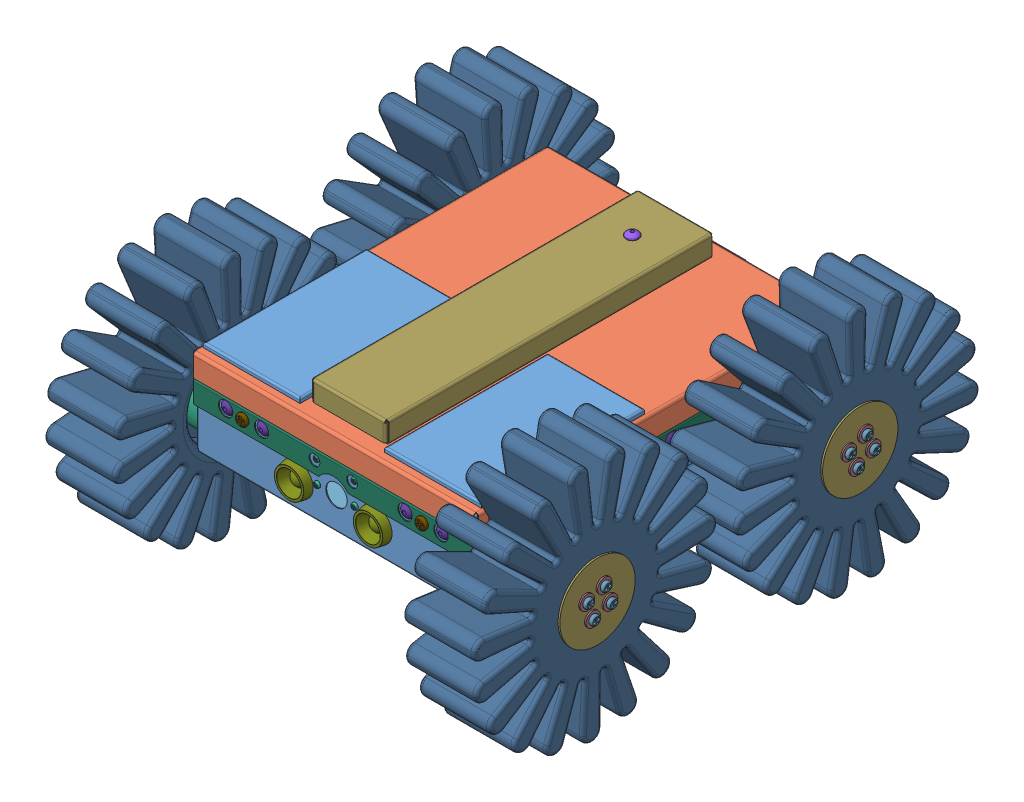
SolidWorks assembly GB0814, configuration Default. Lengths in mm. (continued)
Components (placement in the parent): (continued)
- wheel.assembly-2: wheel.assembly [Default] at (63.2286 -85.6639 -5.4063) x (0 0.437031 0.899447) z (-1 0 0) size (135.84 135.37 44.03)
  - wheel-1: wheel [Default] at (66.6468 86.2072 65.7286) size (135.84 135.37 40.29)
  - wheel.spacer-1: wheel.spacer [Default] at (66.6468 86.2072 79.7286) x (0.629376 -0.777101 0) z (-0.777101 -0.629376 0) size (21 1 21)
  - wheel.flap-1: wheel.flap [Default] at (66.6468 86.2072 106.7286) x (-0.999542 -0.030263 0) z (0 0 -1) size (42 42 1)
  - m3.washer-1: m3.washer [Default] at (69.6683 92.7975 107.5286) x (-0.923728 -0.383049 0) z (0 0 -1) size (8 8 0.8)
  - m3.washer-2: m3.washer [Default] at (60.0564 89.2288 107.5286) x (-0.923728 -0.383049 0) z (0 0 -1) size (8 8 0.8)
  - m3.washer-3: m3.washer [Default] at (63.6252 79.6169 107.5286) x (-0.923728 -0.383049 0) z (0 0 -1) size (8 8 0.8)
  - m3.washer-4: m3.washer [Default] at (73.2371 83.1856 107.5286) x (-0.923728 -0.383049 0) z (0 0 -1) size (8 8 0.8)
  - m3.screw.36mm-1: m3.screw.36mm [Default] at (73.2444 83.2034 107.5286) x (-0.923728 -0.383049 0) z (0 0 -1) size (5.42 5.42 38.08)
  - m3.screw.36mm-2: m3.screw.36mm [Default] at (63.6325 79.6346 107.5286) x (-0.923728 -0.383049 0) z (0 0 -1) size (5.42 5.42 38.08)
  - m3.screw.36mm-3: m3.screw.36mm [Default] at (69.6757 92.8153 107.5286) x (-0.923728 -0.383049 0) z (0 0 -1) size (5.42 5.42 38.08)
  - m3.screw.36mm-4: m3.screw.36mm [Default] at (60.0754 89.232 107.5286) x (-0.815437 0.578846 0) z (0 0 -1) size (5.42 5.42 38.08)
- wheel.assembly-3: wheel.assembly [Default] at (63.2286 -73.2341 108.359) x (0 0.131707 0.991289) z (-1 0 0) size (135.84 135.37 44.03)
  - wheel-1: wheel [Default] at (66.6468 86.2072 65.7286) size (135.84 135.37 40.29)
  - wheel.spacer-1: wheel.spacer [Default] at (66.6468 86.2072 79.7286) x (0.629376 -0.777101 0) z (-0.777101 -0.629376 0) size (21 1 21)
  - wheel.flap-1: wheel.flap [Default] at (66.6468 86.2072 106.7286) x (-0.999542 -0.030263 0) z (0 0 -1) size (42 42 1)
  - m3.washer-1: m3.washer [Default] at (69.6683 92.7975 107.5286) x (-0.923728 -0.383049 0) z (0 0 -1) size (8 8 0.8)
  - m3.washer-2: m3.washer [Default] at (60.0564 89.2288 107.5286) x (-0.923728 -0.383049 0) z (0 0 -1) size (8 8 0.8)
  - m3.washer-3: m3.washer [Default] at (63.6252 79.6169 107.5286) x (-0.923728 -0.383049 0) z (0 0 -1) size (8 8 0.8)
  - m3.washer-4: m3.washer [Default] at (73.2371 83.1856 107.5286) x (-0.923728 -0.383049 0) z (0 0 -1) size (8 8 0.8)
  - m3.screw.36mm-1: m3.screw.36mm [Default] at (73.2444 83.2034 107.5286) x (-0.923728 -0.383049 0) z (0 0 -1) size (5.42 5.42 38.08)
  - m3.screw.36mm-2: m3.screw.36mm [Default] at (63.6325 79.6346 107.5286) x (-0.923728 -0.383049 0) z (0 0 -1) size (5.42 5.42 38.08)
  - m3.screw.36mm-3: m3.screw.36mm [Default] at (69.6757 92.8153 107.5286) x (-0.923728 -0.383049 0) z (0 0 -1) size (5.42 5.42 38.08)
  - m3.screw.36mm-4: m3.screw.36mm [Default] at (60.0754 89.232 107.5286) x (-0.815437 0.578846 0) z (0 0 -1) size (5.42 5.42 38.08)
- wheel.assembly-4: wheel.assembly [Default] at (91.7714 80.2331 108.0959) x (0 -0.996524 -0.08331) z (1 0 0) size (135.84 135.37 44.03)
  - wheel-1: wheel [Default] at (66.6468 86.2072 65.7286) size (135.84 135.37 40.29)
  - wheel.spacer-1: wheel.spacer [Default] at (66.6468 86.2072 79.7286) x (0.629376 -0.777101 0) z (-0.777101 -0.629376 0) size (21 1 21)
  - wheel.flap-1: wheel.flap [Default] at (66.6468 86.2072 106.7286) x (-0.999542 -0.030263 0) z (0 0 -1) size (42 42 1)
  - m3.washer-1: m3.washer [Default] at (69.6683 92.7975 107.5286) x (-0.923728 -0.383049 0) z (0 0 -1) size (8 8 0.8)
  - m3.washer-2: m3.washer [Default] at (60.0564 89.2288 107.5286) x (-0.923728 -0.383049 0) z (0 0 -1) size (8 8 0.8)
  - m3.washer-3: m3.washer [Default] at (63.6252 79.6169 107.5286) x (-0.923728 -0.383049 0) z (0 0 -1) size (8 8 0.8)
  - m3.washer-4: m3.washer [Default] at (73.2371 83.1856 107.5286) x (-0.923728 -0.383049 0) z (0 0 -1) size (8 8 0.8)
  - m3.screw.36mm-1: m3.screw.36mm [Default] at (73.2444 83.2034 107.5286) x (-0.923728 -0.383049 0) z (0 0 -1) size (5.42 5.42 38.08)
  - m3.screw.36mm-2: m3.screw.36mm [Default] at (63.6325 79.6346 107.5286) x (-0.923728 -0.383049 0) z (0 0 -1) size (5.42 5.42 38.08)
  - m3.screw.36mm-3: m3.screw.36mm [Default] at (69.6757 92.8153 107.5286) x (-0.923728 -0.383049 0) z (0 0 -1) size (5.42 5.42 38.08)
  - m3.screw.36mm-4: m3.screw.36mm [Default] at (60.0754 89.232 107.5286) x (-0.815437 0.578846 0) z (0 0 -1) size (5.42 5.42 38.08)
- case.cap-1: case.cap [Default<As Machined>] at (155.5 42 -8.1489) x (-1 0 0) z (0 0 1) size (159 12.5 199)
- cap.fixture-1: cap.fixture [Default] at (145 41.8819 74.9679) x (0 0 1) z (0 -1 0) size (30 10 10)
- cap.fixture-2: cap.fixture [Default] at (10 31.8819 74.9679) x (0 0 1) z (0 1 0) size (30 10 10)
- cap.fixture-3: cap.fixture [Default] at (112.5 31.75 177.0711) x (1 0 0) z (0 1 0) size (30 10 10)
- cap.fixture-4: cap.fixture [Default] at (12.5 31.75 177.0711) x (1 0 0) z (0 1 0) size (30 10 10)
- cap.fixture-5: cap.fixture [Default] at (12.5 41.75 2.636) x (1 0 0) z (0 -1 0) size (30 10 10)
- cap.fixture-6: cap.fixture [Default] at (112.5 41.75 2.636) x (1 0 0) z (0 -1 0) size (30 10 10)
- 4mmx8mm.rivet-1: 4mmx8mm.rivet [Default] at (137.5247 36.75 -6.5519) x (1 0 0) z (0 1 0) size (7.59 9.68 7.59)
- 4mmx8mm.rivet-2: 4mmx8mm.rivet [Default] at (117.5247 36.75 -6.5519) x (1 0 0) z (0 1 0) size (7.59 9.68 7.59)
- 4mmx8mm.rivet-3: 4mmx8mm.rivet [Default] at (37.5247 36.75 -6.5519) x (1 0 0) z (0 1 0) size (7.59 9.68 7.59)
- 4mmx8mm.rivet-4: 4mmx8mm.rivet [Default] at (17.5247 36.75 -6.5519) x (1 0 0) z (0 1 0) size (7.59 9.68 7.59)
- 4mmx8mm.rivet-5: 4mmx8mm.rivet [Default] at (17.5023 36.7254 186.259) x (0.092687 -0.995695 0) z (-0.995695 -0.092687 0) size (7.59 9.68 7.59)
- 4mmx8mm.rivet-6: 4mmx8mm.rivet [Default] at (37.5241 36.7552 186.259) x (0.977227 0.212195 0) z (0.212195 -0.977227 0) size (7.59 9.68 7.59)
- 4mmx8mm.rivet-7: 4mmx8mm.rivet [Default] at (117.5091 36.7271 186.259) x (0.367943 -0.929848 0) z (-0.929848 -0.367943 0) size (7.59 9.68 7.59)
- 4mmx8mm.rivet-8: 4mmx8mm.rivet [Default] at (137.518 36.7332 186.259) x (0.730918 -0.682465 0) z (-0.682465 -0.730918 0) size (7.59 9.68 7.59)
- 4mmx8mm.rivet-9: 4mmx8mm.rivet [Default] at (0.8121 36.9065 79.9679) x (0 1 0) z (0 0 1) size (7.59 9.68 7.59)
- 4mmx8mm.rivet-10: 4mmx8mm.rivet [Default] at (0.8121 36.9065 99.9679) x (0 1 0) z (0 0 1) size (7.59 9.68 7.59)
- 4mmx8mm.rivet-11: 4mmx8mm.rivet [Default] at (154.1879 36.8572 79.9679) x (0 -1 0) z (0 0 1) size (7.59 9.68 7.59)
- 4mmx8mm.rivet-12: 4mmx8mm.rivet [Default] at (154.1879 36.8572 99.9679) x (0 -1 0) z (0 0 1) size (7.59 9.68 7.59)
- m4.screw.15mm-1: m4.screw.15mm [Default] at (127.4864 36.7636 -9.6489) size (6.42 6.42 17)
- m4.screw.15mm-2: m4.screw.15mm [Default] at (27.4864 36.7636 -9.6489) size (6.42 6.42 17)
- m4.screw.15mm-3: m4.screw.15mm [Default] at (27.5073 36.7678 189.3511) x (-0.923728 -0.383049 0) z (0 0 -1) size (6.42 6.42 17)
- m4.screw.15mm-4: m4.screw.15mm [Default] at (127.5073 36.7678 189.3511) x (-0.923728 -0.383049 0) z (0 0 -1) size (6.42 6.42 17)
- m4.screw.15mm-5: m4.screw.15mm [Default] at (-2 36.8954 89.9815) x (0 0 -1) z (1 0 0) size (6.42 6.42 17)
- m4.screw.15mm-6: m4.screw.15mm [Default] at (157 36.8954 89.9543) x (0 0 1) z (-1 0 0) size (6.42 6.42 17)
- solar.panel-2: solar.panel [Default] at (35 42.5 138.8511) size (54 2.5 91)
- solar.panel-3: solar.panel [Default] at (120 42.5 138.8511) size (54 2.5 91)
- solar.panel-4: solar.panel [Default] at (35 42.5 40.8511) size (54 2.5 91)
- solar.panel-5: solar.panel [Default] at (120 42.5 40.8511) size (54 2.5 91)
- case.over.cap-1: case.over.cap [Default<As Machined>] at (155.5 54.4828 -8.1489) x (-1 0 0) z (0 0 1) size (159 12.5 199)
- hinge.p1-1: hinge.p1 [Default] at (107.5 30.4828 -9.6489) x (0 1 0) z (-1 0 0) size (14.5 5 60)
- hinge.p2-1: hinge.p2 [Default] at (47.5588 53.4828 -9.6489) x (0 -1 0) z (1 0 0) size (13.5 5 60)
- solar.panel-6: solar.panel [Default] at (124.5 54.4828 41.3511) x (1 0 0) z (0 0 -1) size (54 2.5 91)
- solar.panel-7: solar.panel [Default] at (124.5 54.4828 138.3511) x (1 0 0) z (0 0 -1) size (54 2.5 91)
- solar.panel-8: solar.panel [Default] at (30.5 54.4828 41.3511) x (1 0 0) z (0 0 -1) size (54 2.5 91)
- solar.panel-9: solar.panel [Default] at (30.5 54.4828 138.3511) x (1 0 0) z (0 0 -1) size (54 2.5 91)
- finger.actuator.p1-1: finger.actuator.p1 [По умолчанию] at (77.5 52.06 170.345) x (-1 0 0) z (0 0.016791 -0.999859) size (15 18 153)
- finger.actuator.p2-1: finger.actuator.p2 [По умолчанию] at (77.5 52.795 126.5769) x (1 0 0) z (0 0.999859 0.016791) size (9 107.09 9)
- actuator.fixture-1: actuator.fixture [Default] at (77.5 42.5 174.8444) size (10.47 13.5 8)
- 4mmx4mm.rivet-1: 4mmx4mm.rivet [Default] at (77.5247 45.6879 174.8444) size (7.59 5.68 7.59)
- self.stop.nut.m4-1: self.stop.nut.m4 [Default] at (72.2634 51.9844 174.8444) x (0 1 0) z (0 0 1) size (9.07 4.5 8.37)
- m4.screw.18-1: m4.screw.18 [Default] at (82.7366 51.998 174.8308) x (0 0 1) z (-1 0 0) size (6.42 6.42 20)
- actuator.fixture.p2-1: actuator.fixture.p2 [Default] at (77.4134 66.2194 22.5916) x (1 0 0) z (0 0 -1) size (7.97 15.47 7)
- actuator.cap-1: actuator.cap [Default] at (77.4966 66.7194 89.5968) x (-1 0 0) z (0 0 1) size (42.47 11.74 182.47)
- 4mmx4mm.rivet-2: 4mmx4mm.rivet [Default] at (77.4381 69.4073 22.5916) size (7.59 5.68 7.59)
- 4mmx4mm.rivet-3: 4mmx4mm.rivet [Default] at (61.8816 51.7949 118.4279) x (0.134133 0 0.990963) z (0.990963 0 -0.134133) size (7.59 5.68 7.59)
- 4mmx4mm.rivet-4: 4mmx4mm.rivet [Default] at (93.0942 51.7949 11.5238) x (-0.837169 0 -0.546944) z (-0.546944 0 0.837169) size (7.59 5.68 7.59)
- 4mmx4mm.rivet-5: 4mmx4mm.rivet [Default] at (93.1116 51.7949 60.8146) x (-0.132721 0 0.991153) z (0.991153 0 0.132721) size (7.59 5.68 7.59)
- 4mmx4mm.rivet-6: 4mmx4mm.rivet [Default] at (93.0968 51.7949 118.3866) x (-0.733507 0 -0.679682) z (-0.679682 0 0.733507) size (7.59 5.68 7.59)
- 4mmx4mm.rivet-7: 4mmx4mm.rivet [Default] at (61.8783 51.7949 167.6809) x (-0.000086 0 1) z (1 0 0.000086) size (7.59 5.68 7.59)
- 4mmx4mm.rivet-8: 4mmx4mm.rivet [Default] at (93.1114 51.7949 167.6318) x (-0.142955 0 -0.989729) z (-0.989729 0 0.142955) size (7.59 5.68 7.59)
- 4mmx4mm.rivet-9: 4mmx4mm.rivet [Default] at (61.8552 51.7949 11.5285) x (-0.935337 0 -0.353759) z (-0.353759 0 0.935337) size (7.59 5.68 7.59)
- 4mmx4mm.rivet-10: 4mmx4mm.rivet [Default] at (61.8545 51.7949 60.7837) x (-0.965731 0 -0.259543) z (-0.259543 0 0.965731) size (7.59 5.68 7.59)
- m4.screw.15mm-8: m4.screw.15mm [Default] at (73.4268 54.5549 22.6051) x (0 0 -1) z (1 0 0) size (6.42 6.42 17)
- self.stop.nut.m4-2: self.stop.nut.m4 [Default] at (81.4 54.5413 22.5916) x (0 -1 0) z (0 0 1) size (9.07 4.5 8.37)
- 3gmodem-1: 3gmodem [Default] at (29.9897 40.5099 123.3049) x (-0.008727 0 0.999962) z (0.999962 0 0.008727) size (28.27 12.78 89.07)
  - Main-1: Main [Default] at (-58.655 5.5101 -11.1836) x (0.999962 0 0.008727) z (-0.008727 0 0.999962) size (27.5 12.78 88.83)
- usb.female-1: usb.female [Default] at (93.717 33.8248 65.8015) x (0 0 1) z (-1 0 0) size (25.4 15.88 44.45)
- USB head-1: USB head [Default] at (59.2512 13.406 52.9571) x (0 0 1) z (-1 0 0) size (77.08 29.38 103.42)
- solar.panel-10: solar.panel [Default] at (27 54.9828 138.8511) size (54 2.5 91)
- solar.panel-11: solar.panel [Default] at (128 54.9828 138.8511) size (54 2.5 91)
- LEDLamp-1: LEDLamp [По умолчанию] at (78.9661 -1.0512 155.0023) x (0 0 1) z (-1 0 0) size (28 25.27 25.27)
  - housing-1: housing [По умолчанию] at (8.0687 22.0512 23.4661) size (28 18 18)
  - ledlampnut-1: ledlampnut [По умолчанию] at (32.0687 22.0512 23.4661) x (0 -0.739986 0.672623) z (-1 0 0) size (17.89 17.89 3)
- LEDLamp-2: LEDLamp [По умолчанию] at (122.9661 -1.0512 155.0023) x (0 0 1) z (-1 0 0) size (28 25.27 25.27)
  - housing-1: housing [По умолчанию] at (8.0687 22.0512 23.4661) size (28 18 18)
  - ledlampnut-1: ledlampnut [По умолчанию] at (32.0687 22.0512 23.4661) x (0 -0.739986 0.672623) z (-1 0 0) size (17.89 17.89 3)
Mates (geometry in assembly coordinates):
- Coincident6: coincident aligned: plane of SM4315R-2 through (17.9812 31.16 7.636) normal (0 1 0); plane of SM4315R-3 through (137.0187 31.16 7.636) normal (0 1 0)
- Coincident7: coincident aligned: plane of SM4315R-2 through (17.9812 10.84 48.276) normal (0 0 1); plane of SM4315R-3 through (137.0187 31.16 48.276) normal (0 0 1)
- Coincident8: coincident aligned: plane of SM4315R-1 through (17.9812 31.16 172.0711) normal (0 1 0); plane of SM4315R-4 through (137.0187 31.16 172.0711) normal (0 1 0)
- Coincident9: coincident aligned: plane of SM4315R-1 through (17.9812 31.16 131.4311) normal (0 0 -1); plane of SM4315R-4 through (137.0187 10.84 131.4311) normal (0 0 -1)
- Coincident10: coincident aligned: plane of SM4315R-3 through (137.0187 31.16 7.636) normal (0 1 0); plane of SM4315R-4 through (137.0187 31.16 172.0711) normal (0 1 0)
- Parallel9: parallel aligned: plane of SM4315R-3 through (137.0187 31.16 7.636) normal (0 1 0); plane of assembly through (0 0 0) normal (0 1 0)
- Parallel10: parallel anti-aligned: plane of SM4315R-2 through (7.4 31.16 48.276) normal (-1 0 0); plane of assembly through (0 0 0) normal (1 0 0)
- Parallel11: parallel anti-aligned: plane of SM4315R-1 through (7.4 10.84 131.4311) normal (-1 0 0); plane of assembly through (0 0 0) normal (1 0 0)
- Parallel12: parallel anti-aligned: plane of case.bottom-1 through (0 0 0) normal (0 1 0); plane of raspberrypi_b_+_(assembly)-1/raspberry_pi_B+_(CI_Board)-1 through (102.9674 12.4 163.6067) normal (0 -1 0)
- Concentric1: concentric aligned: cylinder of SM4315R-2 through (1.4 21 16.636) axis (1 0 0) radius 2.5; cylinder of SM4315R.horn-1 through (1.4 21 16.636) axis (1 0 0) radius 3
- Concentric2: concentric aligned: cylinder of SM4315R-1 through (1.4 21 163.0711) axis (1 0 0) radius 2.5; cylinder of SM4315R.horn-2 through (1.4 21 163.0711) axis (1 0 0) radius 3
- Concentric3: concentric aligned: cylinder of SM4315R-4 through (153.6 21 163.0711) axis (-1 0 0) radius 2.5; cylinder of SM4315R.horn-4 through (153.6 21 163.0711) axis (-1 0 0) radius 3
- Coincident15: coincident anti-aligned: plane of SM4315R-4 through (153.6 21 163.0711) normal (1 0 0); plane of SM4315R.horn-4 through (153.6 21 163.0711) normal (-1 0 0)
- Concentric5: concentric aligned: cylinder of SM4315R-3 through (153.6 21 16.636) axis (-1 0 0) radius 2.5; cylinder of SM4315R.horn-3 through (153.6 21 16.636) axis (-1 0 0) radius 3
- Coincident16: coincident anti-aligned: plane of SM4315R-3 through (153.6 21 16.636) normal (1 0 0); plane of SM4315R.horn-3 through (153.6 21 16.636) normal (-1 0 0)
- Coincident34: coincident aligned: plane of accumulator-3 through (21.0287 7 -0.1494) normal (0 0 -1); plane of accumulator-4 through (78.5703 7 -0.1494) normal (0 0 -1)
- Coincident35: coincident aligned: plane of accumulator-1 through (21.0287 7 180.3909) normal (-1 0 0); plane of accumulator-3 through (21.0287 7 -0.1494) normal (-1 0 0)
- Coincident36: coincident aligned: plane of accumulator-2 through (133.5703 7 180.9066) normal (1 0 0); plane of accumulator-4 through (133.5703 7 -0.1494) normal (1 0 0)
- Coincident42: coincident aligned: plane of flange-1 through (-0.5 21.0015 16.8638) normal (1 0 0); plane of wheel.hub-1 through (-0.5 21 16.636) normal (1 0 0)
- Coincident45: coincident aligned: plane of case.bottom-1 through (-0.5 0 0) normal (-1 0 0); plane of SM4315R.horn-1 through (-0.5 21 16.636) normal (-1 0 0)
- Coincident46: coincident anti-aligned: plane of case.bottom-1 through (-0.5 0 0) normal (-1 0 0); plane of wheel.hub-1 through (-0.5 21 16.636) normal (1 0 0)
- Concentric14: concentric aligned: cylinder of SM4315R.horn-1 through (-0.5 21 16.636) axis (1 0 0) radius 10.45; cylinder of wheel.hub-1 through (-16.5 21 16.636) axis (1 0 0) radius 10.5
- Coincident50: coincident anti-aligned: plane of raspberrypi_b_+_(assembly)-1/raspberry_pi_B+_(bar_180_2x20)-1 through (52.5307 22.5 112.92) normal (0 0 1); plane of pin.2.54.holder-1 through (50.9807 30.75 112.92) normal (0 0 -1)
- Coincident51: coincident anti-aligned: plane of raspberrypi_b_+_(assembly)-1/raspberry_pi_B+_(bar_180_2x20)-1 through (51.8807 22.5 112.92) normal (-1 0 0); plane of pin.2.54.holder-1 through (51.8807 30.75 111.32) normal (1 0 0)
- Coincident52: coincident anti-aligned: plane of raspberrypi_b_+_(assembly)-1/raspberry_pi_B+_(bar_180_2x20)-1 through (54.4457 16.5 158.315) normal (0 1 0); plane of pin.2.54.holder-1 through (52.2307 16.5 112.57) normal (0 -1 0)
- Coincident53: coincident anti-aligned: plane of case.bottom-1 through (0 0 0) normal (1 0 0); plane of self.stop.nut.m3-2 through (0 38 16.636) normal (-1 0 0)
- Coincident54: coincident anti-aligned: plane of case.bottom-1 through (0 0 0) normal (1 0 0); plane of self.stop.nut.m3-4 through (0 4.0031 17.0915) normal (-1 0 0)
- Coincident55: coincident anti-aligned: plane of case.bottom-1 through (0 0 0) normal (1 0 0); plane of self.stop.nut.m3-3 through (0 20.7738 -0.1347) normal (-1 0 0)
- Coincident57: coincident anti-aligned: plane of case.bottom-1 through (0 0 0) normal (1 0 0); plane of self.stop.nut.m3-1 through (0 21.2293 33.8623) normal (-1 0 0)
- Distance13: distance = 10.84 mm: plane of SM4315R-2 through (17.9812 10.84 7.636) normal (0 -1 0); plane of case.bottom-1 through (0 0 0) normal (0 1 0)
- Distance14: distance = 1 mm anti-aligned: plane of case.bottom-1 through (0 0 0) normal (0 1 0); plane of accumulator-2 through (133.5703 1 180.9066) normal (0 -1 0)
- Distance15: distance = 1 mm anti-aligned: plane of accumulator-4 through (78.5703 1 -0.1494) normal (0 -1 0); plane of case.bottom-1 through (0 0 0) normal (0 1 0)
- Distance16: distance = 1 mm anti-aligned: plane of accumulator-3 through (21.0287 1 -0.1494) normal (0 -1 0); plane of case.bottom-1 through (0 0 0) normal (0 1 0)
- Distance17: distance = 1 mm anti-aligned: plane of accumulator-1 through (76.0287 1 180.3909) normal (0 -1 0); plane of case.bottom-1 through (0 0 0) normal (0 1 0)
- Distance18: distance = 15 mm anti-aligned: plane of case.bottom-1 through (0 0.2929 -7.364) normal (0 0 1); plane of SM4315R-2 through (17.9812 10.84 7.636) normal (0 0 -1)
- Distance23: distance = 7.4 mm anti-aligned: plane of case.bottom-1 through (0 0 0) normal (1 0 0); plane of SM4315R-2 through (7.4 31.16 48.276) normal (-1 0 0)
- Distance19: distance = 15 mm anti-aligned: plane of case.bottom-1 through (0 0 187.0711) normal (0 0 -1); plane of SM4315R-1 through (17.9812 31.16 172.0711) normal (0 0 1)
- Distance24: distance = 7.4 mm anti-aligned: plane of case.bottom-1 through (0 0 0) normal (1 0 0); plane of SM4315R-1 through (7.4 10.84 131.4311) normal (-1 0 0)
- Tangent5: tangent anti-aligned: cylinder of wheel.hub-1 through (-16.5 21 16.636) axis (1 0 0) radius 10.5; sphere of ball.4mm-1
- Tangent6: tangent anti-aligned: plane of wheel.hub-1 through (-4.5 21 16.636) normal (1 0 0); unknown of ball.4mm-1
- Concentric28: concentric aligned: cylinder of case.bottom-1 through (1.5 38 16.636) axis (-1 0 0) radius 1.5; cylinder of flange-1 through (-0.5 38 16.636) axis (-1 0 0) radius 1.5
- Concentric29: concentric aligned: cylinder of SM4315R.horn-1 through (-0.5 21 16.636) axis (1 0 0) radius 10.45; cylinder of wheel.hub-1 through (-16.5 21 16.636) axis (1 0 0) radius 10.5
- Lock2: lock: unknown of case.bottom-1; unknown of flange-1
- Concentric30: concentric anti-aligned: cylinder of flange-1 through (-0.5 38 16.636) axis (-1 0 0) radius 1.5; cylinder of self.stop.nut.m3-2 through (0 38 16.636) axis (1 0 0) radius 1.5
- Concentric31: concentric anti-aligned: cylinder of flange-1 through (-0.5 20.7738 -0.1347) axis (-1 0 0) radius 1.5; cylinder of self.stop.nut.m3-3 through (0 20.7738 -0.1347) axis (1 0 0) radius 1.5
- Concentric32: concentric anti-aligned: cylinder of flange-1 through (-0.5 21.2293 33.8623) axis (-1 0 0) radius 1.5; cylinder of self.stop.nut.m3-1 through (0 21.2293 33.8623) axis (1 0 0) radius 1.5
- Concentric33: concentric anti-aligned: cylinder of flange-1 through (-0.5 4.0031 17.0915) axis (-1 0 0) radius 1.5; cylinder of self.stop.nut.m3-4 through (0 4.0031 17.0915) axis (1 0 0) radius 1.5
- Concentric34: concentric aligned: cylinder of flange-1 through (-0.5 4.0031 17.0915) axis (-1 0 0) radius 1.5; cylinder of m3.screw.18mm-3 through (4.75 4.0031 17.0915) axis (-1 0 0) radius 1.5
- Concentric35: concentric aligned: cylinder of flange-1 through (-0.5 21.2293 33.8623) axis (-1 0 0) radius 1.5; cylinder of m3.screw.18mm-5 through (4.75 21.2293 33.8623) axis (-1 0 0) radius 1.5
- Concentric36: concentric aligned: cylinder of flange-1 through (-0.5 38 16.636) axis (-1 0 0) radius 1.5; cylinder of m3.screw.18mm-2 through (4.75 38 16.636) axis (-1 0 0) radius 1.5
- Concentric37: concentric aligned: cylinder of flange-1 through (-0.5 20.7738 -0.1347) axis (-1 0 0) radius 1.5; cylinder of m3.screw.18mm-4 through (4.75 20.7738 -0.1347) axis (-1 0 0) radius 1.5
- Coincident58: coincident aligned: plane of flange-1 through (-15.5 21.0015 16.8638) normal (-1 0 0); plane of m3.screw.18mm-2 through (-15.5 38 16.636) normal (-1 0 0)
- Coincident59: coincident aligned: plane of flange-1 through (-15.5 21.0015 16.8638) normal (-1 0 0); plane of m3.screw.18mm-5 through (-15.5 21.2293 33.8623) normal (-1 0 0)
- Coincident60: coincident aligned: plane of flange-1 through (-15.5 21.0015 16.8638) normal (-1 0 0); plane of m3.screw.18mm-3 through (-15.5 4.0031 17.0915) normal (-1 0 0)
- Coincident61: coincident aligned: plane of flange-1 through (-15.5 21.0015 16.8638) normal (-1 0 0); plane of m3.screw.18mm-4 through (-15.5 20.7738 -0.1347) normal (-1 0 0)
- Concentric38: concentric aligned: cylinder of wheel.hub-1 through (-0.5 21 16.636) axis (-1 0 0) radius 1.5; cylinder of m3.screw.30mm-6 through (15.75 21 16.636) axis (-1 0 0) radius 1.5
- Coincident62: coincident aligned: plane of wheel.hub-1 through (-16.5 21 16.636) normal (-1 0 0); plane of m3.screw.30mm-6 through (-16.5 21 16.636) normal (-1 0 0)
- Tangent7: tangent anti-aligned: plane of flange-1 through (-12.5 21.0015 16.8638) normal (1 0 0); unknown of ball.4mm-19
- Tangent8: tangent aligned: cylinder of flange-1 through (-12.5 21.0015 16.8638) axis (1 0 0) radius 14.5; unknown of ball.4mm-19
- Concentric43: concentric aligned: cylinder of SM4315R.horn-2 through (1.4 21 163.0711) axis (-1 0 0) radius 1.5; cylinder of wheel.hub-2 through (-0.5 21 163.0711) axis (-1 0 0) radius 1.5
- Concentric44: concentric aligned: cylinder of SM4315R.horn-2 through (4.9 27.9309 165.1983) axis (-1 0 0) radius 1; cylinder of wheel.hub-2 through (-0.5 27.9309 165.1983) axis (-1 0 0) radius 1
- Coincident65: coincident anti-aligned: plane of SM4315R.horn-2 through (-0.5 21 163.0711) normal (-1 0 0); plane of wheel.hub-2 through (-0.5 21 163.0711) normal (1 0 0)
- Concentric45: concentric aligned: cylinder of wheel.hub-2 through (-0.5 21 163.0711) axis (-1 0 0) radius 1.5; cylinder of m3.screw.30mm-7 through (15.75 21 163.0711) axis (-1 0 0) radius 1.5
- Coincident66: coincident aligned: plane of wheel.hub-2 through (-16.5 21 163.0711) normal (-1 0 0); plane of m3.screw.30mm-7 through (-16.5 21 163.0711) normal (-1 0 0)
- Tangent9: tangent anti-aligned: cylinder of wheel.hub-2 through (-16.5 21 163.0711) axis (1 0 0) radius 10.5; unknown of ball.4mm-37
- Tangent10: tangent anti-aligned: plane of wheel.hub-2 through (-4.5 21 163.0711) normal (1 0 0); unknown of ball.4mm-37
- Tangent11: tangent anti-aligned: plane of wheel.hub-2 through (-8.5 21 163.0711) normal (-1 0 0); unknown of ball.4mm-55
- Tangent12: tangent anti-aligned: cylinder of wheel.hub-2 through (-16.5 21 163.0711) axis (1 0 0) radius 10.5; unknown of ball.4mm-55
- Concentric46: concentric aligned: cylinder of case.bottom-1 through (0 38 163.0711) axis (-1 0 0) radius 1.5; cylinder of flange-2 through (-0.5 38 163.0711) axis (-1 0 0) radius 1.5
- Concentric47: concentric aligned: cylinder of case.bottom-1 through (0 4 163.0711) axis (-1 0 0) radius 1.5; cylinder of flange-2 through (-0.5 4 163.0711) axis (-1 0 0) radius 1.5
- Coincident67: coincident anti-aligned: plane of case.bottom-1 through (-0.5 0 0) normal (-1 0 0); plane of flange-2 through (-0.5 21 163.0711) normal (1 0 0)
- Concentric48: concentric aligned: cylinder of flange-2 through (-0.5 21 146.0711) axis (-1 0 0) radius 1.5; cylinder of m3.screw.18mm-7 through (4.75 21 146.0711) axis (-1 0 0) radius 1.5
- Concentric49: concentric aligned: cylinder of flange-2 through (-0.5 4 163.0711) axis (-1 0 0) radius 1.5; cylinder of m3.screw.18mm-6 through (4.75 4 163.0711) axis (-1 0 0) radius 1.5
- Concentric50: concentric aligned: cylinder of flange-2 through (-0.5 38 163.0711) axis (-1 0 0) radius 1.5; cylinder of m3.screw.18mm-8 through (4.75 38 163.0711) axis (-1 0 0) radius 1.5
- Concentric51: concentric aligned: cylinder of flange-2 through (-0.5 21 180.0711) axis (-1 0 0) radius 1.5; cylinder of m3.screw.18mm-9 through (4.75 21 180.0711) axis (-1 0 0) radius 1.5
- Coincident68: coincident aligned: plane of flange-2 through (-15.5 21 163.0711) normal (-1 0 0); plane of m3.screw.18mm-7 through (-15.5 21 146.0711) normal (-1 0 0)
- Coincident69: coincident aligned: plane of flange-2 through (-15.5 21 163.0711) normal (-1 0 0); plane of m3.screw.18mm-8 through (-15.5 38 163.0711) normal (-1 0 0)
- Coincident70: coincident aligned: plane of flange-2 through (-15.5 21 163.0711) normal (-1 0 0); plane of m3.screw.18mm-9 through (-15.5 21 180.0711) normal (-1 0 0)
- Coincident71: coincident aligned: plane of flange-2 through (-15.5 21 163.0711) normal (-1 0 0); plane of m3.screw.18mm-6 through (-15.5 4 163.0711) normal (-1 0 0)
- Concentric52: concentric aligned: cylinder of SM4315R.horn-4 through (153.6 21 163.0711) axis (1 0 0) radius 1.5; cylinder of wheel.hub-3 through (155.5 21 163.0711) axis (1 0 0) radius 1.5
- Concentric53: concentric aligned: cylinder of SM4315R.horn-4 through (150.1 17.7804 156.5752) axis (1 0 0) radius 1; cylinder of wheel.hub-3 through (155.5 17.7804 156.5752) axis (1 0 0) radius 1
- Coincident72: coincident anti-aligned: plane of SM4315R.horn-4 through (155.5 21 163.0711) normal (1 0 0); plane of wheel.hub-3 through (155.5 21 163.0711) normal (-1 0 0)
- Concentric54: concentric anti-aligned: cylinder of m3.screw.18mm-6 through (4.75 4 163.0711) axis (-1 0 0) radius 1.5; cylinder of self.stop.nut.m3-8 through (0 4 163.0711) axis (1 0 0) radius 1.5
- Concentric55: concentric anti-aligned: cylinder of m3.screw.18mm-7 through (4.75 21 146.0711) axis (-1 0 0) radius 1.5; cylinder of self.stop.nut.m3-7 through (0 21 146.0711) axis (1 0 0) radius 1.5
- Concentric56: concentric anti-aligned: cylinder of m3.screw.18mm-9 through (4.75 21 180.0711) axis (-1 0 0) radius 1.5; cylinder of self.stop.nut.m3-6 through (0 21 180.0711) axis (1 0 0) radius 1.5
- Concentric57: concentric anti-aligned: cylinder of m3.screw.18mm-8 through (4.75 38 163.0711) axis (-1 0 0) radius 1.5; cylinder of self.stop.nut.m3-5 through (0 38 163.0711) axis (1 0 0) radius 1.5
- Coincident73: coincident anti-aligned: plane of case.bottom-1 through (0 0 0) normal (1 0 0); plane of self.stop.nut.m3-6 through (0 21 180.0711) normal (-1 0 0)
- Coincident74: coincident anti-aligned: plane of case.bottom-1 through (0 0 0) normal (1 0 0); plane of self.stop.nut.m3-8 through (0 4 163.0711) normal (-1 0 0)
- Coincident75: coincident anti-aligned: plane of case.bottom-1 through (0 0 0) normal (1 0 0); plane of self.stop.nut.m3-5 through (0 38 163.0711) normal (-1 0 0)
- Coincident76: coincident anti-aligned: plane of case.bottom-1 through (0 0 0) normal (1 0 0); plane of self.stop.nut.m3-7 through (0 21 146.0711) normal (-1 0 0)
- Concentric58: concentric anti-aligned: cylinder of SM4315R.horn-2 through (4.9 14.0691 160.9438) axis (-1 0 0) radius 1; cylinder of m2.screw-4 through (-6.6 14.0691 160.9438) axis (1 0 0) radius 1
- Concentric59: concentric anti-aligned: cylinder of SM4315R.horn-2 through (4.9 23.1273 156.1402) axis (-1 0 0) radius 1; cylinder of m2.screw-2 through (-6.6 23.1273 156.1402) axis (1 0 0) radius 1
- Concentric60: concentric anti-aligned: cylinder of SM4315R.horn-2 through (4.9 18.8727 170.002) axis (-1 0 0) radius 1; cylinder of m2.screw-1 through (-6.6 18.8727 170.002) axis (1 0 0) radius 1
- Concentric61: concentric anti-aligned: cylinder of SM4315R.horn-2 through (4.9 27.9309 165.1983) axis (-1 0 0) radius 1; cylinder of m2.screw-3 through (-6.6 27.9309 165.1983) axis (1 0 0) radius 1
- Lock4: lock: unknown of case.bottom-1; unknown of SM4315R-1
- Lock5: lock: unknown of case.bottom-1; unknown of flange-2
- Coincident77: coincident anti-aligned: plane of SM4315R.horn-2 through (1.4 21 163.0711) normal (1 0 0); plane of m2.screw-2 through (1.4 23.1324 156.1217) normal (-1 0 0)
- Coincident78: coincident anti-aligned: plane of SM4315R.horn-2 through (1.4 21 163.0711) normal (1 0 0); plane of m2.screw-3 through (1.4 27.944 165.1843) normal (-1 0 0)
- Coincident79: coincident anti-aligned: plane of SM4315R.horn-2 through (1.4 21 163.0711) normal (1 0 0); plane of m2.screw-4 through (1.4 14.0879 160.948) normal (-1 0 0)
- Coincident80: coincident anti-aligned: plane of SM4315R.horn-2 through (1.4 21 163.0711) normal (1 0 0); plane of m2.screw-1 through (1.4 18.8918 170.0041) normal (-1 0 0)
- Coincident81: coincident anti-aligned: plane of SM4315R.horn-1 through (1.4 21 16.636) normal (1 0 0); plane of m2.screw-7 through (1.4 21.0136 23.8724) normal (-1 0 0)
- Coincident82: coincident anti-aligned: plane of SM4315R.horn-1 through (1.4 21 16.636) normal (1 0 0); plane of m2.screw-8 through (1.4 28.2636 16.6224) normal (-1 0 0)
- Coincident83: coincident anti-aligned: plane of SM4315R.horn-1 through (1.4 21 16.636) normal (1 0 0); plane of m2.screw-6 through (1.4 21.0136 9.3724) normal (-1 0 0)
- Coincident84: coincident anti-aligned: plane of SM4315R.horn-1 through (1.4 21 16.636) normal (1 0 0); plane of m2.screw-5 through (1.4 13.7636 16.6224) normal (-1 0 0)
- Concentric62: concentric anti-aligned: cylinder of SM4315R.horn-1 through (4.9 13.75 16.636) axis (-1 0 0) radius 1; cylinder of m2.screw-5 through (-6.6 13.75 16.636) axis (1 0 0) radius 1
- Concentric63: concentric anti-aligned: cylinder of SM4315R.horn-1 through (4.9 21 9.386) axis (-1 0 0) radius 1; cylinder of m2.screw-6 through (-6.6 21 9.386) axis (1 0 0) radius 1
- Concentric64: concentric anti-aligned: cylinder of SM4315R.horn-1 through (4.9 21 23.886) axis (-1 0 0) radius 1; cylinder of m2.screw-7 through (-6.6 21 23.886) axis (1 0 0) radius 1
- Concentric66: concentric anti-aligned: cylinder of SM4315R.horn-1 through (4.9 28.25 16.636) axis (-1 0 0) radius 1; cylinder of m2.screw-8 through (-6.6 28.25 16.636) axis (1 0 0) radius 1
- Lock6: lock: unknown of case.bottom-1; unknown of SM4315R-2
- Tangent13: tangent anti-aligned: cylinder of wheel.hub-3 through (171.5 21 163.0711) axis (-1 0 0) radius 10.5; unknown of ball.4mm-73
- Tangent14: tangent anti-aligned: plane of wheel.hub-3 through (159.5 21 163.0711) normal (-1 0 0); unknown of ball.4mm-73
- Distance20: distance = 7.4 mm anti-aligned: plane of case.bottom-1 through (155 0 0) normal (-1 0 0); plane of SM4315R-4 through (147.6 31.16 131.4311) normal (1 0 0)
- Lock7: lock: unknown of case.bottom-1; unknown of SM4315R-4
- Tangent15: tangent anti-aligned: cylinder of wheel.hub-3 through (171.5 21 163.0711) axis (-1 0 0) radius 10.5; unknown of ball.4mm-96
- Tangent16: tangent anti-aligned: plane of wheel.hub-3 through (163.5 21 163.0711) normal (1 0 0); unknown of ball.4mm-96
- Concentric67: concentric aligned: cylinder of wheel.hub-3 through (163.5 21 163.0711) axis (-1 0 0) radius 13; cylinder of flange-3 through (167.5 21 163.0711) axis (-1 0 0) radius 14.5
- Concentric68: concentric anti-aligned: cylinder of case.bottom-1 through (155.5 38 163.0711) axis (-1 0 0) radius 1.5; cylinder of flange-3 through (155.5 38 163.0711) axis (1 0 0) radius 1.5
- Coincident85: coincident anti-aligned: plane of case.bottom-1 through (155.5 0 0) normal (1 0 0); plane of flange-3 through (155.5 21 163.0711) normal (-1 0 0)
- Concentric69: concentric aligned: cylinder of wheel.hub-3 through (155.5 21 163.0711) axis (1 0 0) radius 1.5; cylinder of m3.screw.30mm-8 through (139.25 21 163.0711) axis (1 0 0) radius 1.5
- Concentric70: concentric aligned: cylinder of flange-3 through (155.5 38 163.0711) axis (1 0 0) radius 1.5; cylinder of m3.screw.18mm-10 through (150.25 38 163.0711) axis (1 0 0) radius 1.5
- Concentric71: concentric aligned: cylinder of flange-3 through (155.5 21 180.0711) axis (1 0 0) radius 1.5; cylinder of m3.screw.18mm-11 through (150.25 21 180.0711) axis (1 0 0) radius 1.5
- Concentric72: concentric aligned: cylinder of flange-3 through (155.5 4 163.0711) axis (1 0 0) radius 1.5; cylinder of m3.screw.18mm-13 through (150.25 4 163.0711) axis (1 0 0) radius 1.5
- Concentric73: concentric aligned: cylinder of flange-3 through (155.5 21 146.0711) axis (1 0 0) radius 1.5; cylinder of m3.screw.18mm-12 through (150.25 21 146.0711) axis (1 0 0) radius 1.5
- Coincident86: coincident aligned: plane of wheel.hub-3 through (171.5 21 163.0711) normal (1 0 0); plane of m3.screw.30mm-8 through (171.5 21 163.0711) normal (1 0 0)
- Coincident87: coincident aligned: plane of flange-3 through (170.5 21 163.0711) normal (1 0 0); plane of m3.screw.18mm-11 through (170.5 21 180.0711) normal (1 0 0)
- Coincident88: coincident aligned: plane of flange-3 through (170.5 21 163.0711) normal (1 0 0); plane of m3.screw.18mm-10 through (170.5 38 163.0711) normal (1 0 0)
- Coincident89: coincident aligned: plane of flange-3 through (170.5 21 163.0711) normal (1 0 0); plane of m3.screw.18mm-12 through (170.5 21 146.0711) normal (1 0 0)
- Coincident90: coincident aligned: plane of flange-3 through (170.5 21 163.0711) normal (1 0 0); plane of m3.screw.18mm-13 through (170.5 4 163.0711) normal (1 0 0)
- Concentric74: concentric anti-aligned: cylinder of m3.screw.18mm-13 through (150.25 4 163.0711) axis (1 0 0) radius 1.5; cylinder of self.stop.nut.m3-9 through (155 4 163.0711) axis (-1 0 0) radius 1.5
- Concentric75: concentric anti-aligned: cylinder of m3.screw.18mm-11 through (150.25 21 180.0711) axis (1 0 0) radius 1.5; cylinder of self.stop.nut.m3-10 through (155 21 180.0711) axis (-1 0 0) radius 1.5
- Concentric76: concentric anti-aligned: cylinder of m3.screw.18mm-12 through (150.25 21 146.0711) axis (1 0 0) radius 1.5; cylinder of self.stop.nut.m3-12 through (155 21 146.0711) axis (-1 0 0) radius 1.5
- Concentric77: concentric anti-aligned: cylinder of m3.screw.18mm-10 through (150.25 38 163.0711) axis (1 0 0) radius 1.5; cylinder of self.stop.nut.m3-11 through (155 38 163.0711) axis (-1 0 0) radius 1.5
- Coincident91: coincident anti-aligned: plane of case.bottom-1 through (155 0 0) normal (-1 0 0); plane of self.stop.nut.m3-11 through (155 38 163.0711) normal (1 0 0)
- Coincident92: coincident anti-aligned: plane of case.bottom-1 through (155 0 0) normal (-1 0 0); plane of self.stop.nut.m3-9 through (155 4 163.0711) normal (1 0 0)
- Coincident93: coincident anti-aligned: plane of case.bottom-1 through (155 0 0) normal (-1 0 0); plane of self.stop.nut.m3-12 through (155 21 146.0711) normal (1 0 0)
- Coincident94: coincident anti-aligned: plane of case.bottom-1 through (155 0 0) normal (-1 0 0); plane of self.stop.nut.m3-10 through (155 21 180.0711) normal (1 0 0)
- Coincident99: coincident anti-aligned: plane of SM4315R.horn-4 through (153.6 21 163.0711) normal (-1 0 0); plane of m2.screw-9 through (153.6 24.2061 169.5534) normal (1 0 0)
- Concentric79: concentric anti-aligned: cylinder of SM4315R.horn-4 through (150.1 24.2196 169.5669) axis (1 0 0) radius 1; cylinder of m2.screw-9 through (161.6 24.2196 169.5669) axis (-1 0 0) radius 1
- Concentric80: concentric anti-aligned: cylinder of SM4315R.horn-4 through (150.1 14.5041 166.2907) axis (1 0 0) radius 1; cylinder of m2.screw-10 through (161.6 14.5041 166.2907) axis (-1 0 0) radius 1
- Coincident100: coincident anti-aligned: plane of SM4315R.horn-4 through (153.6 21 163.0711) normal (-1 0 0); plane of m2.screw-10 through (153.6 14.4933 166.3066) normal (1 0 0)
- Coincident101: coincident anti-aligned: plane of SM4315R.horn-4 through (153.6 21 163.0711) normal (-1 0 0); plane of m2.screw-11 through (153.6 27.5095 159.865) normal (1 0 0)
- Concentric81: concentric anti-aligned: cylinder of SM4315R.horn-4 through (150.1 27.4959 159.8514) axis (1 0 0) radius 1; cylinder of m2.screw-11 through (161.6 27.4959 159.8514) axis (-1 0 0) radius 1
- Coincident102: coincident anti-aligned: plane of SM4315R.horn-4 through (153.6 21 163.0711) normal (-1 0 0); plane of m2.screw-12 through (153.6 17.7939 156.5888) normal (1 0 0)
- Concentric82: concentric anti-aligned: cylinder of SM4315R.horn-4 through (150.1 17.7804 156.5752) axis (1 0 0) radius 1; cylinder of m2.screw-12 through (161.6 17.7804 156.5752) axis (-1 0 0) radius 1
- Distance22: distance = 7.4 mm anti-aligned: plane of SM4315R-3 through (147.6 10.84 48.276) normal (1 0 0); plane of case.bottom-1 through (155 0 0) normal (-1 0 0)
- Lock8: lock: unknown of case.bottom-1; unknown of SM4315R-3
- Coincident103: coincident anti-aligned: plane of SM4315R.horn-3 through (155.5 21 16.636) normal (1 0 0); plane of wheel.hub-4 through (155.5 21 16.636) normal (-1 0 0)
- Concentric83: concentric aligned: cylinder of SM4315R.horn-3 through (153.6 21 16.636) axis (1 0 0) radius 1.5; cylinder of wheel.hub-4 through (155.5 21 16.636) axis (1 0 0) radius 1.5
- Concentric84: concentric aligned: cylinder of SM4315R.horn-3 through (150.1 27.8192 14.174) axis (1 0 0) radius 1; cylinder of wheel.hub-4 through (155.5 27.8192 14.174) axis (1 0 0) radius 1
- Tangent17: tangent anti-aligned: cylinder of wheel.hub-4 through (171.5 21 16.636) axis (-1 0 0) radius 10.5; unknown of ball.4mm-115
- Tangent18: tangent anti-aligned: plane of wheel.hub-4 through (159.5 21 16.636) normal (-1 0 0); unknown of ball.4mm-115
- Tangent19: tangent anti-aligned: cylinder of wheel.hub-4 through (171.5 21 16.636) axis (-1 0 0) radius 10.5; unknown of ball.4mm-116
- Tangent20: tangent anti-aligned: plane of wheel.hub-4 through (163.5 21 16.636) normal (1 0 0); unknown of ball.4mm-116
- Concentric85: concentric aligned: cylinder of wheel.hub-4 through (163.5 21 16.636) axis (-1 0 0) radius 13; cylinder of flange-4 through (167.5 21 16.636) axis (-1 0 0) radius 14.5
- Concentric86: concentric anti-aligned: cylinder of case.bottom-1 through (155.5 38 16.636) axis (-1 0 0) radius 1.5; cylinder of flange-4 through (155.5 38 16.636) axis (1 0 0) radius 1.5
- Coincident104: coincident anti-aligned: plane of case.bottom-1 through (155.5 0 0) normal (1 0 0); plane of flange-4 through (155.5 21 16.636) normal (-1 0 0)
- Lock9: lock: unknown of case.bottom-1; unknown of flange-4
- Concentric87: concentric aligned: cylinder of wheel.hub-4 through (155.5 21 16.636) axis (1 0 0) radius 1.5; cylinder of m3.screw.30mm-9 through (139.25 21 16.636) axis (1 0 0) radius 1.5
- Concentric88: concentric aligned: cylinder of flange-4 through (155.5 21 33.636) axis (1 0 0) radius 1.5; cylinder of m3.screw.18mm-14 through (150.25 21 33.636) axis (1 0 0) radius 1.5
- Concentric89: concentric aligned: cylinder of flange-4 through (155.5 4 16.636) axis (1 0 0) radius 1.5; cylinder of m3.screw.18mm-15 through (150.25 4 16.636) axis (1 0 0) radius 1.5
- Concentric90: concentric aligned: cylinder of flange-4 through (155.5 38 16.636) axis (1 0 0) radius 1.5; cylinder of m3.screw.18mm-16 through (150.25 38 16.636) axis (1 0 0) radius 1.5
- Concentric91: concentric aligned: cylinder of flange-4 through (155.5 21 -0.364) axis (1 0 0) radius 1.5; cylinder of m3.screw.18mm-17 through (150.25 21 -0.364) axis (1 0 0) radius 1.5
- Coincident105: coincident aligned: plane of wheel.hub-4 through (171.5 21 16.636) normal (1 0 0); plane of m3.screw.30mm-9 through (171.5 21 16.636) normal (1 0 0)
- Coincident106: coincident aligned: plane of flange-4 through (170.5 21 16.636) normal (1 0 0); plane of m3.screw.18mm-16 through (170.5 38 16.636) normal (1 0 0)
- Coincident107: coincident aligned: plane of flange-4 through (170.5 21 16.636) normal (1 0 0); plane of m3.screw.18mm-14 through (170.5 21 33.636) normal (1 0 0)
- Coincident108: coincident aligned: plane of flange-4 through (170.5 21 16.636) normal (1 0 0); plane of m3.screw.18mm-15 through (170.5 4 16.636) normal (1 0 0)
- Coincident109: coincident aligned: plane of flange-4 through (170.5 21 16.636) normal (1 0 0); plane of m3.screw.18mm-17 through (170.5 21 -0.364) normal (1 0 0)
- Coincident110: coincident anti-aligned: plane of SM4315R.horn-3 through (153.6 21 16.636) normal (-1 0 0); plane of m2.screw-13 through (153.6 14.1944 19.1117) normal (1 0 0)
- Coincident111: coincident anti-aligned: plane of SM4315R.horn-3 through (153.6 21 16.636) normal (-1 0 0); plane of m2.screw-14 through (153.6 18.5516 9.8305) normal (1 0 0)
- Coincident112: coincident anti-aligned: plane of SM4315R.horn-3 through (153.6 21 16.636) normal (-1 0 0); plane of m2.screw-15 through (153.6 27.8327 14.1876) normal (1 0 0)
- Coincident113: coincident anti-aligned: plane of SM4315R.horn-3 through (153.6 21 16.636) normal (-1 0 0); plane of m2.screw-16 through (153.6 23.4756 23.4688) normal (1 0 0)
- Concentric92: concentric anti-aligned: cylinder of SM4315R.horn-3 through (150.1 14.1808 19.0981) axis (1 0 0) radius 1; cylinder of m2.screw-13 through (161.6 14.1808 19.0981) axis (-1 0 0) radius 1
- Concentric93: concentric anti-aligned: cylinder of SM4315R.horn-3 through (150.1 18.538 9.8169) axis (1 0 0) radius 1; cylinder of m2.screw-14 through (161.6 18.538 9.8169) axis (-1 0 0) radius 1
- Concentric94: concentric anti-aligned: cylinder of SM4315R.horn-3 through (150.1 27.8192 14.174) axis (1 0 0) radius 1; cylinder of m2.screw-15 through (161.6 27.8192 14.174) axis (-1 0 0) radius 1
- Concentric95: concentric anti-aligned: cylinder of SM4315R.horn-3 through (150.1 23.462 23.4552) axis (1 0 0) radius 1; cylinder of m2.screw-16 through (161.6 23.462 23.4552) axis (-1 0 0) radius 1
- Coincident114: coincident anti-aligned: plane of case.bottom-1 through (155 0 0) normal (-1 0 0); plane of self.stop.nut.m3-13 through (155 4 16.636) normal (1 0 0)
- Coincident115: coincident anti-aligned: plane of case.bottom-1 through (155 0 0) normal (-1 0 0); plane of self.stop.nut.m3-14 through (155 21 33.636) normal (1 0 0)
- Coincident116: coincident anti-aligned: plane of case.bottom-1 through (155 0 0) normal (-1 0 0); plane of self.stop.nut.m3-15 through (155 21 -0.364) normal (1 0 0)
- Coincident117: coincident anti-aligned: plane of case.bottom-1 through (155 0 0) normal (-1 0 0); plane of self.stop.nut.m3-16 through (155 38 16.636) normal (1 0 0)
- Concentric97: concentric anti-aligned: cylinder of m3.screw.18mm-15 through (150.25 4 16.636) axis (1 0 0) radius 1.5; cylinder of self.stop.nut.m3-13 through (155 4 16.636) axis (-1 0 0) radius 1.5
- Concentric98: concentric anti-aligned: cylinder of m3.screw.18mm-14 through (150.25 21 33.636) axis (1 0 0) radius 1.5; cylinder of self.stop.nut.m3-14 through (155 21 33.636) axis (-1 0 0) radius 1.5
- Concentric99: concentric anti-aligned: cylinder of m3.screw.18mm-17 through (150.25 21 -0.364) axis (1 0 0) radius 1.5; cylinder of self.stop.nut.m3-15 through (155 21 -0.364) axis (-1 0 0) radius 1.5
- Concentric100: concentric anti-aligned: cylinder of m3.screw.18mm-16 through (150.25 38 16.636) axis (1 0 0) radius 1.5; cylinder of self.stop.nut.m3-16 through (155 38 16.636) axis (-1 0 0) radius 1.5
- Coincident118: coincident anti-aligned: plane of case.bottom-1 through (0 0 0) normal (0 1 0); plane of servo.fixture-1 through (135.0187 0 27.956) normal (0 -1 0)
- Coincident119: coincident anti-aligned: plane of SM4315R-3 through (137.0187 21 17.796) normal (-1 0 0); plane of servo.fixture-1 through (137.0187 19 27.956) normal (1 0 0)
- Concentric103: concentric anti-aligned: cylinder of servo.fixture-1 through (153.0188 15.92 52.086) axis (-1 0 0) radius 1.5; cylinder of m3.screw.10mm-8 through (129.4 15.92 52.086) axis (1 0 0) radius 1.5
- Concentric104: concentric anti-aligned: cylinder of servo.fixture-1 through (153.0188 26.08 52.086) axis (-1 0 0) radius 1.5; cylinder of m3.screw.10mm-7 through (129.4 26.08 52.086) axis (1 0 0) radius 1.5
- Concentric105: concentric anti-aligned: cylinder of servo.fixture-1 through (153.0188 15.92 3.826) axis (-1 0 0) radius 1.5; cylinder of m3.screw.10mm-6 through (129.4 15.92 3.826) axis (1 0 0) radius 1.5
- Concentric106: concentric anti-aligned: cylinder of servo.fixture-1 through (153.0188 26.08 3.826) axis (-1 0 0) radius 1.5; cylinder of m3.screw.10mm-5 through (129.4 26.08 3.826) axis (1 0 0) radius 1.5
- Coincident122: coincident anti-aligned: plane of SM4315R-3 through (139.4 21 17.796) normal (1 0 0); plane of m3.screw.10mm-5 through (139.4 26.0936 3.8124) normal (-1 0 0)
- Coincident123: coincident anti-aligned: plane of SM4315R-3 through (139.4 21 17.796) normal (1 0 0); plane of m3.screw.10mm-6 through (139.4 15.9336 3.8124) normal (-1 0 0)
- Coincident125: coincident anti-aligned: plane of SM4315R-3 through (139.4 21 17.796) normal (1 0 0); plane of m3.screw.10mm-8 through (139.4 15.9336 52.0724) normal (-1 0 0)
- Coincident126: coincident anti-aligned: plane of SM4315R-3 through (139.4 21 17.796) normal (1 0 0); plane of m3.screw.10mm-7 through (139.4 26.0945 52.0734) normal (-1 0 0)
- Concentric107: concentric anti-aligned: cylinder of m3.screw.10mm-8 through (129.4 15.92 52.086) axis (1 0 0) radius 1.5; cylinder of self.stop.nut.m3-21 through (135.0187 15.92 52.086) axis (-1 0 0) radius 1.5
- Coincident127: coincident anti-aligned: plane of servo.fixture-1 through (135.0187 19 27.956) normal (-1 0 0); plane of self.stop.nut.m3-21 through (135.0187 15.92 52.086) normal (1 0 0)
- Concentric108: concentric anti-aligned: cylinder of m3.screw.10mm-7 through (129.4 26.08 52.086) axis (1 0 0) radius 1.5; cylinder of self.stop.nut.m3-19 through (135.0187 26.08 52.086) axis (-1 0 0) radius 1.5
- Coincident128: coincident anti-aligned: plane of servo.fixture-1 through (135.0187 19 27.956) normal (-1 0 0); plane of self.stop.nut.m3-19 through (135.0187 26.08 52.086) normal (1 0 0)
- Concentric109: concentric anti-aligned: cylinder of m3.screw.10mm-5 through (129.4 26.08 3.826) axis (1 0 0) radius 1.5; cylinder of self.stop.nut.m3-18 through (135.0187 26.08 3.826) axis (-1 0 0) radius 1.5
- Coincident129: coincident anti-aligned: plane of servo.fixture-1 through (135.0187 19 27.956) normal (-1 0 0); plane of self.stop.nut.m3-18 through (135.0187 26.08 3.826) normal (1 0 0)
- Concentric110: concentric anti-aligned: cylinder of m3.screw.10mm-6 through (129.4 15.92 3.826) axis (1 0 0) radius 1.5; cylinder of self.stop.nut.m3-20 through (135.0187 15.92 3.826) axis (-1 0 0) radius 1.5
- Coincident130: coincident anti-aligned: plane of servo.fixture-1 through (135.0187 19 27.956) normal (-1 0 0); plane of self.stop.nut.m3-20 through (135.0187 15.92 3.826) normal (1 0 0)
